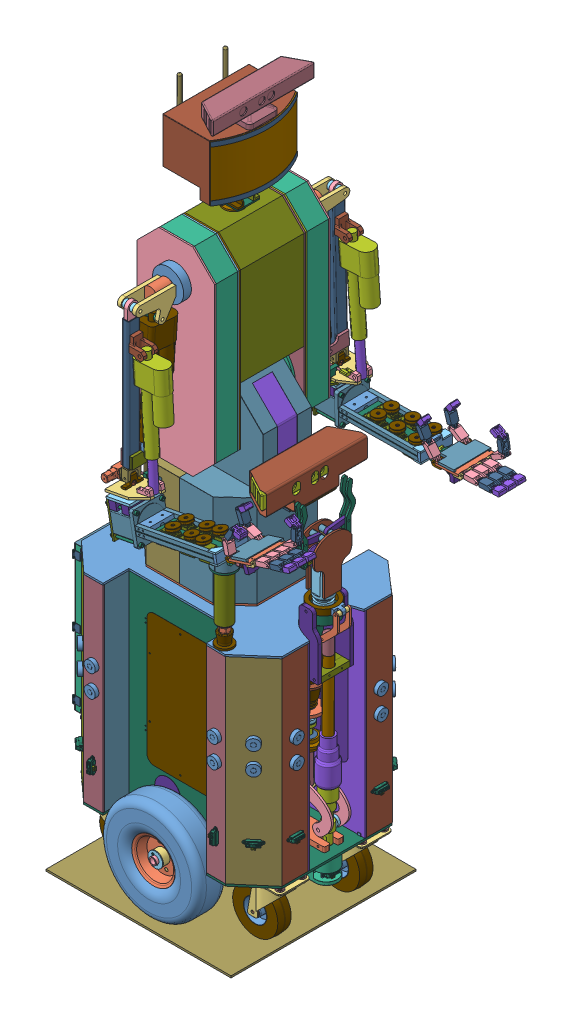
SolidWorks assembly sorbot, configuration По умолчанию. Lengths in mm. (continued)
Components (placement in the parent): (continued)
- man1.drive1-1: man1.drive1 [По умолчанию] at (-119.3768 640.728 -141.6211) x (0.999934 0 -0.01146) z (0 1 0) size (50 50 148.25)
- body.tilit.planetary.drive.fixture.p1-1: body.tilit.planetary.drive.fixture.p1 [По умолчанию] at (-119.3768 612.7934 -141.6211) size (85 10 85)
- body.tilit.planetary.drive.fixture.p2-1: body.tilit.planetary.drive.fixture.p2 [По умолчанию] at (-119.3768 622.7934 -141.6211) size (85 4 85)
- tilt.thread.rod.fixture.2-2: tilt.thread.rod.fixture.2 [По умолчанию] at (-119.3768 793.5591 -141.6211) x (-0.837169 0 -0.546944) z (-0.546944 0 0.837169) size (40 26 40)
- body.tilit.planetary.drive.fixture.p3-1: body.tilit.planetary.drive.fixture.p3 [По умолчанию] at (-119.3768 695.728 -141.6211) size (68 8 68)
- body.tilit.planetary.drive.fixture.p4-1: body.tilit.planetary.drive.fixture.p4 [По умолчанию] at (-119.3768 753.9526 -141.6211) x (0.997546 0 -0.070011) z (0.070011 0 0.997546) size (70 9 70)
- body.tilit.planetary.drive.fixture.p5-1: body.tilit.planetary.drive.fixture.p5 [По умолчанию] at (-148.8664 612.7934 -141.6211) size (5 157 5)
- m6.nut-13: m6.nut [По умолчанию] at (-148.8664 613.2934 -141.6211) size (10 5.5 11.55)
- body.tilit.planetary.drive.fixture.p5-2: body.tilit.planetary.drive.fixture.p5 [По умолчанию] at (-89.8872 612.7934 -141.6211) size (5 157 5)
- body.tilit.planetary.drive.fixture.p5-3: body.tilit.planetary.drive.fixture.p5 [По умолчанию] at (-119.3768 612.7934 -112.1315) size (5 157 5)
- body.tilit.planetary.drive.fixture.p5-4: body.tilit.planetary.drive.fixture.p5 [По умолчанию] at (-119.3768 612.7934 -171.1107) size (5 157 5)
- m6.nut-14: m6.nut [По умолчанию] at (-89.8872 613.2934 -141.6211) size (10 5.5 11.55)
- m6.nut-15: m6.nut [По умолчанию] at (-119.3768 613.2934 -171.1107) x (0.598875 0 -0.800843) z (0.800843 0 0.598875) size (10 5.5 11.55)
- m6.nut-16: m6.nut [По умолчанию] at (-119.3768 613.2934 -112.1315) x (-0.286054 0 -0.958214) z (0.958214 0 -0.286054) size (10 5.5 11.55)
- m6.nut-17: m6.nut [По умолчанию] at (-119.3768 768.4526 -112.1315) x (-0.837169 0 -0.546944) z (-0.546944 0 0.837169) size (10 5.5 11.55)
- m6.nut-18: m6.nut [По умолчанию] at (-89.8872 768.4526 -141.6211) x (-0.837169 0 -0.546944) z (-0.546944 0 0.837169) size (10 5.5 11.55)
- m6.nut-19: m6.nut [По умолчанию] at (-119.3768 768.4526 -171.1107) x (-0.837169 0 -0.546944) z (-0.546944 0 0.837169) size (10 5.5 11.55)
- m6.nut-20: m6.nut [По умолчанию] at (-148.8664 768.4526 -141.6211) x (-0.837169 0 -0.546944) z (-0.546944 0 0.837169) size (10 5.5 11.55)
- m6.nut-21: m6.nut [По умолчанию] at (-29.5996 1324.99 9.9014) x (-0.526603 0.850111 0) z (0 0 1) size (10 5.5 11.55)
- m6.6.50mm-1: m6.6.50mm [По умолчанию] at (4.3029 1345.9909 9.9014) x (0.525089 -0.847668 0.075763) z (-0.039897 0.064407 0.997126) size (10 56 10)
- m4.nut-1: m4.nut [По умолчанию] at (-35.3987 1340.8364 4.6679) x (1 0 0) z (0 -1 0) size (6.86 5 7.92)
- m4.nut-2: m4.nut [По умолчанию] at (-103.2224 997.8992 -35.7442) x (1 0 0) z (0 -1 0) size (6.86 5 7.92)
- arm.rotate-1: arm.rotate [По умолчанию] at (22.4782 854.2475 144.4763) x (0 0 1) z (-0.185706 0.982605 0) size (85.26 111.5 91.5)
  - SY85STH65-2808A-1: SY85STH65-2808A [По умолчанию] at (-4.2017 8.56 0) size (85.26 96.5 85)
  - m6.6.80mm-1: m6.6.80mm [По умолчанию] at (-39.0017 18.56 -34.8) size (10 86 10)
  - m6.6.80mm-2: m6.6.80mm [По умолчанию] at (30.5983 18.56 34.8) size (10 86 10)
  - m6.6.80mm-3: m6.6.80mm [По умолчанию] at (30.5983 18.56 -34.8) size (10 86 10)
  - m6.6.80mm-4: m6.6.80mm [По умолчанию] at (-39.0017 18.56 34.8) size (10 86 10)
  - arm.rotate.p2-2: arm.rotate.p2 [По умолчанию] at (-46.7017 -46.44 42.5) x (1 0 0) z (0 -1 0) size (85 91.5 5)
  - m6.nut-1: m6.nut [По умолчанию] at (30.5983 -56.94 34.8) size (10 5.5 11.55)
  - m6.nut-2: m6.nut [По умолчанию] at (-39.0017 -56.94 -34.8) size (10 5.5 11.55)
  - m6.nut-3: m6.nut [По умолчанию] at (-39.0017 -56.94 34.8) size (10 5.5 11.55)
  - m6.nut-4: m6.nut [По умолчанию] at (30.5983 -56.94 -34.8) size (10 5.5 11.55)
  - arm.rotate.p1-2: arm.rotate.p1 [По умолчанию] at (-4.2017 8.56 38) x (1 0 0) z (0 -1 0) size (85 21 20)
  - arm.rotate.p1-3: arm.rotate.p1 [По умолчанию] at (-4.2017 -26.44 38) x (1 0 0) z (0 -1 0) size (85 21 20)
- arm.rotate.p8-1: arm.rotate.p8 [По умолчанию] at (-48.9081 912.5039 130.5417) x (-0.185706 0.982605 0) z (0 0 1) size (25 12 48)
- arm.rotate.p9-1: arm.rotate.p9 [По умолчанию] at (42.4949 859.0482 172.7746) x (0.982605 0.185706 0) z (0 0 1) size (30 10 65)
- arm.rotate.p9-2: arm.rotate.p9 [По умолчанию] at (72.3444 862.6542 172.7746) x (-0.982605 -0.185706 0) z (0 0 1) size (30 10 65)
- arm.elbow.rotate.p1-1: arm.elbow.rotate.p1 [По умолчанию] at (-55.7977 924.3811 168.7746) x (-0.185706 0.982605 0) z (0 0 -1) size (21.9 27.89 71.5)
- arm.rotate.p6-1: arm.rotate.p6 [По умолчанию] at (20.223 919.4631 140.2746) x (0 0 1) z (-0.982605 -0.185706 0) size (85 6 102)
- arm.rotate.p7-1: arm.rotate.p7 [По умолчанию] at (81.3033 937.1131 170.2746) x (-0.185706 0.982605 0) z (0 0 -1) size (16 36 10)
- arm.rotate.p7-2: arm.rotate.p7 [По умолчанию] at (81.3033 937.1131 140.2746) x (-0.185706 0.982605 0) z (0 0 -1) size (16 36 10)
- arm.rotate.p10-1: arm.rotate.p10 [По умолчанию] at (-37.1666 892.8424 182.7746) x (0 0 -1) z (0.982605 0.185706 0) size (85 6 65)
- arm.elbow.rotate.bearing-1: arm.elbow.rotate.bearing [По умолчанию] at (-7.5173 911.1932 140.056) x (-0.183128 -0.03461 0.98248) z (-0.96539 -0.182453 -0.18637) size (61.4 10 61.4)
  - arm.elbow.rotate.bearing.p1-1: arm.elbow.rotate.bearing.p1 [По умолчанию] at (0.2225 -3.7755 0) size (61.4 4.5 61.4)
  - ball.10mm-1: ball.10mm [По умолчанию] at (0.0947 -1.5255 -24.7664) size (10 10 10)
  - ball.10mm-2: ball.10mm [По умолчанию] at (-9.9677 -1.5255 -22.5733) x (0.913545 0 -0.406737) z (0.406737 0 0.913545) size (10 10 10)
  - ball.10mm-3: ball.10mm [По умолчанию] at (-18.2681 -1.5255 -16.477) x (0.669131 0 -0.743145) z (0.743145 0 0.669131) size (10 10 10)
  - ball.10mm-4: ball.10mm [По умолчанию] at (-23.3713 -1.5255 -7.5317) x (0.309017 0 -0.951057) z (0.951057 0 0.309017) size (10 10 10)
  - ball.10mm-5: ball.10mm [По умолчанию] at (-24.3949 -1.5255 2.7159) x (-0.104528 0 -0.994522) z (0.994522 0 -0.104528) size (10 10 10)
  - ball.10mm-6: ball.10mm [По умолчанию] at (-21.162 -1.5255 12.4939) x (-0.5 0 -0.866025) z (0.866025 0 -0.5) size (10 10 10)
  - ball.10mm-7: ball.10mm [По умолчанию] at (-14.2315 -1.5255 20.1116) x (-0.809017 0 -0.587785) z (0.587785 0 -0.809017) size (10 10 10)
  - ball.10mm-8: ball.10mm [По умолчанию] at (-4.8018 -1.5255 24.2518) x (-0.978148 0 -0.207912) z (0.207912 0 -0.978148) size (10 10 10)
  - ball.10mm-9: ball.10mm [По умолчанию] at (5.4967 -1.5255 24.1987) x (-0.978148 0 0.207912) z (-0.207912 0 -0.978148) size (10 10 10)
  - ball.10mm-10: ball.10mm [По умолчанию] at (14.8832 -1.5255 19.9614) x (-0.809017 0 0.587785) z (-0.587785 0 -0.809017) size (10 10 10)
  - ball.10mm-11: ball.10mm [По умолчанию] at (21.7347 -1.5255 12.2726) x (-0.5 0 0.866025) z (-0.866025 0 -0.5) size (10 10 10)
  - ball.10mm-12: ball.10mm [По умолчанию] at (24.8666 -1.5255 2.4617) x (-0.104528 0 0.994522) z (-0.994522 0 -0.104528) size (10 10 10)
  - ball.10mm-13: ball.10mm [По умолчанию] at (23.7373 -1.5255 -7.7748) x (0.309017 0 0.951057) z (-0.951057 0 0.309017) size (10 10 10)
  - ball.10mm-14: ball.10mm [По умолчанию] at (18.542 -1.5255 -16.6669) x (0.669131 0 0.743145) z (-0.743145 0 0.669131) size (10 10 10)
  - ball.10mm-15: ball.10mm [По умолчанию] at (10.1792 -1.5255 -22.6772) x (0.913545 0 0.406737) z (-0.406737 0 0.913545) size (10 10 10)
- arm.elbow.rotate.p3-1: arm.elbow.rotate.p3 [По умолчанию] at (-6.3462 904.7735 140.2746) x (0.982605 0.185706 0) z (0 0 1) size (36.4 9 36.4)
- arm.elbow.rotate.p4-1: arm.elbow.rotate.p4 [По умолчанию] at (-6.3462 904.7735 140.2746) x (0.982605 0.185706 0) z (0 0 1) size (22 7 22)
- bolt.m8.short-1: bolt.m8.short [По умолчанию] at (-3.7463 891.017 140.2746) x (0.982605 0.185706 0) z (0 0 1) size (12.8 43 12.8)
- m8.nut-1: m8.nut [По умолчанию] at (-9.2247 920.0039 140.2746) x (0.979774 0.185171 -0.075859) z (0.07454 0.014088 0.997119) size (14.97 7 13.53)
- arm.rotate.p11-1: arm.rotate.p11 [По умолчанию] at (-41.1593 913.9684 141.7746) x (-0.185706 0.982605 0) z (0 0 -1) size (24 14 44)
- arm.elbow.rotate.p5-1: arm.elbow.rotate.p5 [По умолчанию] at (-37.816 927.7795 114.7746) x (-0.0817 0.432291 -0.898025) z (0.982605 0.185706 0) size (5 5 75)
- arm.elbow.rotate.p6-1: arm.elbow.rotate.p6 [По умолчанию] at (39.7316 938.238 120.2746) x (0 0 1) z (-0.982685 -0.185282 0) size (21 8 17.99)
- arm.elbow.rotate.p11-1: arm.elbow.rotate.p11 [По умолчанию] at (-1.3122 934.6785 114.7746) x (0 0 -1) z (0.982605 0.185706 0) size (29.5 27.93 10)
- arm.elbow.rotate.p12-1: arm.elbow.rotate.p12 [По умолчанию] at (0.0407 905.9806 81.7746) x (0.589563 0.111424 0.8) z (-0.786084 -0.148565 0.6) size (29 4.5 14)
- arm.elbow.rotate.p13-1: arm.elbow.rotate.p13 [По умолчанию] at (-28.3338 929.5716 114.7746) x (-0.185706 0.982605 0) z (0 0 1) size (9 12 9)
- arm.elbow.rotate.p14-1: arm.elbow.rotate.p14 [По умолчанию] at (-41.599 927.0645 114.7746) x (0 0 -1) z (0.982605 0.185706 0) size (18 18 10)
- palm.tilt.p1-1: palm.tilt.p1 [По умолчанию] at (76.6621 839.8086 140.4246) x (0.185706 -0.982605 0) z (0 0 1) size (36.5 37.1 24.8)
- palm.drives.fixture-2: palm.drives.fixture [По умолчанию] at (72.6077 850.4915 150.4246) x (0.982605 0.185706 0) z (0 0 -1) size (30.05 15 65)
- palm.lift.p2-2: palm.lift.p2 [По умолчанию] at (97.1945 857.1737 140.4246) x (0.033136 -0.175327 -0.983952) z (0.982605 0.185706 0) size (5 5 158)
- palm.drive.thread.fixture.p2-1: palm.drive.thread.fixture.p2 [По умолчанию] at (87.8616 855.4098 140.4246) x (-0.05957 0.315194 0.947156) z (0.982605 0.185706 0) size (11.8 11.8 25)
- m3x8-1: m3x8 [По умолчанию] at (92.8919 850.6734 142.3172) x (0.982605 0.185707 0) z (0.05957 -0.315194 -0.947156) size (5.3 6.85 5.3)
- m3x8-2: m3x8 [По умолчанию] at (101.0372 852.2128 142.3172) x (0.982605 0.185707 0) z (0.05957 -0.315194 -0.947156) size (5.3 6.85 5.3)
- palm.drive.thread.fixture-1: palm.drive.thread.fixture [По умолчанию] at (254.7288 885.7804 140.4246) x (0 0 -1) z (-0.982605 -0.185706 0) size (30 34 7)
- palm.lift.fixture-1: palm.lift.fixture [По умолчанию] at (260.6332 900.2751 126.1211) x (0 0 -1) z (0.185706 -0.982605 0) size (30 17 12)
- palm.lift.fixture.p2-1: palm.lift.fixture.p2 [По умолчанию] at (287.8736 901.2786 140.2746) x (0 0 1) z (-0.950223 -0.311571 0) size (26 12.5 30)
- PALM.LIFT.THREAD.FIXTURE.P3-1: PALM.LIFT.THREAD.FIXTURE.P3 [По умолчанию] at (131.0658 873.7522 140.2958) x (-0.982605 -0.185706 0) z (0 0 1) size (20 14 10)
- palm.lift.drive.nut-1: palm.lift.drive.nut [По умолчанию] at (168.1531 870.5844 140.4246) x (0.124167 -0.656989 -0.743604) z (0.982605 0.185706 0) size (12 12 16)
- palm.lift.nut.fixture-1: palm.lift.nut.fixture [По умолчанию] at (174.1569 881.8961 145.4246) x (0 0 -1) z (-0.982605 -0.185706 0) size (10 28 10)
- palm.lift.nut.fixture-2: palm.lift.nut.fixture [По умолчанию] at (174.1569 881.8961 135.4246) x (0 0 1) z (0.982605 0.185706 0) size (10 28 10)
- palm.lift.p4-1: palm.lift.p4 [По умолчанию] at (168.591 857.4974 140.4246) x (0 0 -1) z (0.982605 0.185706 0) size (4 4 120)
- palm.lift.fixture.p6-1: palm.lift.fixture.p6 [По умолчанию] at (276.6776 877.9252 140.4246) x (0 0 -1) z (0.982605 0.185706 0) size (12 12 20.44)
- palm.lift.fixture.p7-1: palm.lift.fixture.p7 [По умолчанию] at (292.1321 880.846 138.4246) x (0.730069 0.683374 0) z (0 0 1) size (27 9 4)
- m6.washer-1: m6.washer [По умолчанию] at (284.4317 914.5677 140.506) x (0.950223 0.311571 0.000222) z (-0.000211 -0.000069 1) size (18 1.7 18)
- m6.washer-2: m6.washer [По умолчанию] at (289.4791 899.1741 140.506) x (-0.950223 -0.311571 -0.000219) z (-0.000208 -0.000068 1) size (18 1.7 18)
- m6.washer-3: m6.washer [По умолчанию] at (286.8308 907.251 140.506) x (0.950223 0.311571 0.000222) z (-0.000211 -0.000069 1) size (18 1.7 18)
- palm.lift.on-palm.fixture-2: palm.lift.on-palm.fixture [По умолчанию] at (300.1799 895.8423 140.2746) x (0 0 -1) z (0.950223 0.311571 0) size (26 23.89 8)
- palm.lift.p1-1: palm.lift.p1 [По умолчанию] at (338.412 919.9816 174.4917) x (0.950144 0.311545 0.012888) z (-0.311571 0.950223 0) size (36.5 37.1 24.8)
- palm.drive.thread.fixture.p2-2: palm.drive.thread.fixture.p2 [По умолчанию] at (325.9934 915.9097 160.372) x (-0.999321 0.034794 -0.0121) z (0.012247 0.004016 -0.999917) size (11.8 11.8 25)
- palm.tilit.fixture-1: palm.tilit.fixture [По умолчанию] at (336.6565 929.587 176.5089) x (0.012247 0.004016 -0.999917) z (-0.950144 -0.311545 -0.012888) size (12 17 18)
- palm.tilit.p8-1: palm.tilit.p8 [По умолчанию] at (326.1771 915.9699 145.3733) x (-0.999829 0.013918 -0.01219) z (0.012247 0.004016 -0.999917) size (5 5 57)
- palm.tilit.p9-1: palm.tilit.p9 [По умолчанию] at (336.3842 931.6025 91.2066) x (-0.950144 -0.311545 -0.012888) z (-0.012247 -0.004016 0.999917) size (23.81 15.6 6)
- palm.tilit.p10-1: palm.tilit.p10 [По умолчанию] at (303.1082 912.5882 153.2746) x (0 0 -1) z (0.950223 0.311571 0) size (26 8.5 15)
- palm.tilit.p11-1: palm.tilit.p11 [По умолчанию] at (326.5434 916.09 115.4643) x (0.950144 0.311545 0.012888) z (-0.012247 -0.004016 0.999917) size (17.95 8 10)
- palm.tilit.p12-1: palm.tilit.p12 [По умолчанию] at (317.7933 904.2485 140.2746) x (0.070018 0.022958 -0.997282) z (0.94764 0.310724 0.073685) size (29 4 9)
- arm.rotate.p6-2: arm.rotate.p6 [По умолчанию] at (17.2833 914.2431 -421.887) x (-0.005195 -0.022106 0.999742) z (-0.99991 -0.012267 -0.005467) size (85 6 102)
- arm.rotate.p8-2: arm.rotate.p8 [По умолчанию] at (-52.6122 919.605 -432.1343) x (-0.012385 0.99968 0.022041) z (-0.005195 -0.022106 0.999742) size (25 12 48)
- arm.rotate.p7-3: arm.rotate.p7 [По умолчанию] at (80.4988 921.0176 -421.4088) x (-0.012385 0.99968 0.022041) z (0.005195 0.022106 -0.999742) size (16 36 10)
- arm.rotate.p7-4: arm.rotate.p7 [По умолчанию] at (80.343 920.3544 -391.4165) x (-0.012385 0.99968 0.022041) z (0.005195 0.022106 -0.999742) size (16 36 10)
- bolt.m8.short-2: bolt.m8.short [По умолчанию] at (-11.2814 892.2812 -422.5211) x (0.999923 0.012406 -0.000807) z (0.00108 -0.022029 0.999757) size (12.8 43 12.8)
- m8.nut-2: m8.nut [По умолчанию] at (-11.6234 919.8874 -421.9124) x (0.559915 -0.011329 0.828472) z (-0.828457 -0.022602 0.559596) size (14.97 7 13.53)
- arm.elbow.rotate.bearing-2: arm.elbow.rotate.bearing [По умолчанию] at (-11.6907 910.4164 -422.2454) x (0.829913 -0.002018 0.557889) z (-0.557755 -0.025201 0.829623) size (61.4 10 61.4)
  - arm.elbow.rotate.bearing.p1-1: arm.elbow.rotate.bearing.p1 [По умолчанию] at (0.2225 -3.7755 0) size (61.4 4.5 61.4)
  - ball.10mm-1: ball.10mm [По умолчанию] at (0.0947 -1.5255 -24.7664) size (10 10 10)
  - ball.10mm-2: ball.10mm [По умолчанию] at (-9.9677 -1.5255 -22.5733) x (0.913545 0 -0.406737) z (0.406737 0 0.913545) size (10 10 10)
  - ball.10mm-3: ball.10mm [По умолчанию] at (-18.2681 -1.5255 -16.477) x (0.669131 0 -0.743145) z (0.743145 0 0.669131) size (10 10 10)
  - ball.10mm-4: ball.10mm [По умолчанию] at (-23.3713 -1.5255 -7.5317) x (0.309017 0 -0.951057) z (0.951057 0 0.309017) size (10 10 10)
  - ball.10mm-5: ball.10mm [По умолчанию] at (-24.3949 -1.5255 2.7159) x (-0.104528 0 -0.994522) z (0.994522 0 -0.104528) size (10 10 10)
  - ball.10mm-6: ball.10mm [По умолчанию] at (-21.162 -1.5255 12.4939) x (-0.5 0 -0.866025) z (0.866025 0 -0.5) size (10 10 10)
  - ball.10mm-7: ball.10mm [По умолчанию] at (-14.2315 -1.5255 20.1116) x (-0.809017 0 -0.587785) z (0.587785 0 -0.809017) size (10 10 10)
  - ball.10mm-8: ball.10mm [По умолчанию] at (-4.8018 -1.5255 24.2518) x (-0.978148 0 -0.207912) z (0.207912 0 -0.978148) size (10 10 10)
  - ball.10mm-9: ball.10mm [По умолчанию] at (5.4967 -1.5255 24.1987) x (-0.978148 0 0.207912) z (-0.207912 0 -0.978148) size (10 10 10)
  - ball.10mm-10: ball.10mm [По умолчанию] at (14.8832 -1.5255 19.9614) x (-0.809017 0 0.587785) z (-0.587785 0 -0.809017) size (10 10 10)
  - ball.10mm-11: ball.10mm [По умолчанию] at (21.7347 -1.5255 12.2726) x (-0.5 0 0.866025) z (-0.866025 0 -0.5) size (10 10 10)
  - ball.10mm-12: ball.10mm [По умолчанию] at (24.8666 -1.5255 2.4617) x (-0.104528 0 0.994522) z (-0.994522 0 -0.104528) size (10 10 10)
  - ball.10mm-13: ball.10mm [По умолчанию] at (23.7373 -1.5255 -7.7748) x (0.309017 0 0.951057) z (-0.951057 0 0.309017) size (10 10 10)
  - ball.10mm-14: ball.10mm [По умолчанию] at (18.542 -1.5255 -16.6669) x (0.669131 0 0.743145) z (-0.743145 0 0.669131) size (10 10 10)
  - ball.10mm-15: ball.10mm [По умолчанию] at (10.1792 -1.5255 -22.6772) x (0.913545 0 0.406737) z (-0.406737 0 0.913545) size (10 10 10)
- arm.elbow.rotate.p4-2: arm.elbow.rotate.p4 [По умолчанию] at (-11.4253 903.8925 -422.2651) x (0.756023 0.023788 -0.654112) z (0.654428 -0.008562 0.756076) size (22 7 22)
- arm.elbow.rotate.p3-2: arm.elbow.rotate.p3 [По умолчанию] at (-11.4253 903.8925 -422.2651) x (0.999923 0.012396 -0.000381) z (0.000654 -0.022034 0.999757) size (36.4 9 36.4)
- arm.rotate.p10-2: arm.rotate.p10 [По умолчанию] at (-43.7015 904.4334 -464.9318) x (-0.005195 -0.022106 0.999742) z (0.99991 0.012267 0.005467) size (85 6 65)
- arm.rotate-2: arm.rotate [По умолчанию] at (8.1724 849.0496 -419.1732) x (-0.005195 -0.022106 0.999742) z (-0.012385 0.99968 0.022041) size (85.26 111.5 91.5)
  - SY85STH65-2808A-1: SY85STH65-2808A [По умолчанию] at (-4.2017 8.56 0) size (85.26 96.5 85)
  - m6.6.80mm-1: m6.6.80mm [По умолчанию] at (-39.0017 18.56 -34.8) size (10 86 10)
  - m6.6.80mm-2: m6.6.80mm [По умолчанию] at (30.5983 18.56 34.8) size (10 86 10)
  - m6.6.80mm-3: m6.6.80mm [По умолчанию] at (30.5983 18.56 -34.8) size (10 86 10)
  - m6.6.80mm-4: m6.6.80mm [По умолчанию] at (-39.0017 18.56 34.8) size (10 86 10)
  - arm.rotate.p2-2: arm.rotate.p2 [По умолчанию] at (-46.7017 -46.44 42.5) x (1 0 0) z (0 -1 0) size (85 91.5 5)
  - m6.nut-1: m6.nut [По умолчанию] at (30.5983 -56.94 34.8) size (10 5.5 11.55)
  - m6.nut-2: m6.nut [По умолчанию] at (-39.0017 -56.94 -34.8) size (10 5.5 11.55)
  - m6.nut-3: m6.nut [По умолчанию] at (-39.0017 -56.94 34.8) size (10 5.5 11.55)
  - m6.nut-4: m6.nut [По умолчанию] at (30.5983 -56.94 -34.8) size (10 5.5 11.55)
  - arm.rotate.p1-2: arm.rotate.p1 [По умолчанию] at (-4.2017 8.56 38) x (1 0 0) z (0 -1 0) size (85 21 20)
  - arm.rotate.p1-3: arm.rotate.p1 [По умолчанию] at (-4.2017 -26.44 38) x (1 0 0) z (0 -1 0) size (85 21 20)
- arm.rotate.p9-3: arm.rotate.p9 [По умолчанию] at (59.0931 848.0507 -390.6251) x (-0.99991 -0.012267 -0.005467) z (-0.005195 -0.022106 0.999742) size (30 10 65)
- arm.rotate.p9-4: arm.rotate.p9 [По умолчанию] at (29.0711 849.682 -390.745) x (0.99991 0.012267 0.005467) z (-0.005195 -0.022106 0.999742) size (30 10 65)
- arm.rotate.p11.mirr-1: arm.rotate.p11.mirr [По умолчанию] at (-44.3413 918.5492 -379.6011) x (-0.012385 0.99968 0.022041) z (0.005195 0.022106 -0.999742) size (24 14 44)
- arm.elbow.rotate.p1-2: arm.elbow.rotate.p1 [По умолчанию] at (-56.5709 932.0381 -450.3776) x (0.012299 -0.999907 -0.005858) z (-0.005395 -0.005924 0.999968) size (21.9 27.89 71.5)
- arm.elbow.rotate.p6.mirr-1: arm.elbow.rotate.p6.mirr [По умолчанию] at (20.3416 928.6659 -401.5471) x (0.005195 0.022106 -0.999742) z (0.99991 0.012267 0.005467) size (21 8 17.99)
- arm.elbow.rotate.p13-2: arm.elbow.rotate.p13 [По умолчанию] at (-28.5648 932.0653 -396.2246) x (0.012299 -0.999907 -0.005858) z (0.005395 0.005924 -0.999968) size (9 12 9)
- arm.elbow.rotate.p14-2: arm.elbow.rotate.p14 [По умолчанию] at (-42.4135 931.8954 -396.3003) x (0.005872 -0.033224 -0.999431) z (0.99991 0.012267 0.005467) size (18 18 10)
- arm.elbow.rotate.p5-2: arm.elbow.rotate.p5 [По умолчанию] at (-38.5639 931.9427 -396.2793) x (0.005872 -0.033224 -0.999431) z (0.99991 0.012267 0.005467) size (5 5 75)
- arm.elbow.rotate.p11-2: arm.elbow.rotate.p11 [По умолчанию] at (8.5819 932.5211 -396.0215) x (-0.005195 -0.022106 0.999742) z (-0.99991 -0.012267 -0.005467) size (29.5 27.93 10)
- arm.elbow.rotate.p12-2: arm.elbow.rotate.p12 [По умолчанию] at (-5.2424 903.6993 -363.7222) x (0.604102 0.025046 -0.796513) z (0.796811 -0.00345 0.604219) size (29 4.5 14)
- palm.drives.fixture-3: palm.drives.fixture [По умолчанию] at (57.358 836.5241 -413.2447) x (0.99991 0.012267 0.005467) z (0.005195 0.022106 -0.999742) size (30.05 15 65)
- palm.tilt.p1-2: palm.tilt.p1 [По умолчанию] at (59.5491 825.5233 -423.4792) x (0.012385 -0.99968 -0.022041) z (-0.005195 -0.022106 0.999742) size (36.5 37.1 24.8)
- palm.drive.thread.fixture.p2-3: palm.drive.thread.fixture.p2 [По умолчанию] at (73.3338 838.9402 -423.1109) x (0.002801 0.207624 -0.978205) z (0.99991 0.012267 0.005467) size (11.8 11.8 25)
- palm.lift.p2-3: palm.lift.p2 [По умолчанию] at (85.2879 839.0868 -423.0455) x (0.006111 -0.053098 -0.998571) z (0.99991 0.012267 0.005467) size (5 5 158)
- palm.lift.drive.nut-2: palm.lift.drive.nut [По умолчанию] at (152.3766 839.9099 -422.6787) x (-0.003006 -0.192356 0.981321) z (0.99991 0.012267 0.005467) size (12 12 16)
- palm.lift.nut.fixture-3: palm.lift.nut.fixture [По умолчанию] at (160.2261 849.8943 -417.4158) x (0.005195 0.022106 -0.999742) z (-0.99991 -0.012267 -0.005467) size (10 28 10)
- palm.lift.nut.fixture-4: palm.lift.nut.fixture [По умолчанию] at (160.278 850.1154 -427.4132) x (-0.005195 -0.022106 0.999742) z (0.99991 0.012267 0.005467) size (10 28 10)
- palm.lift.p4-2: palm.lift.p4 [По умолчанию] at (150.9783 826.9543 -422.9724) x (-0.009526 0.934752 -0.355174) z (0.99991 0.012267 0.005467) size (4 4 120)
- palm.lift.fixture-2: palm.lift.fixture [По умолчанию] at (251.2934 853.4367 -436.1728) x (0.005195 0.022106 -0.999742) z (0.012385 -0.99968 -0.022041) size (30 17 12)
- palm.lift.fixture.p2-2: palm.lift.fixture.p2 [По умолчанию] at (278.3444 848.1669 -421.9915) x (-0.005195 -0.022106 0.999742) z (-0.998179 -0.059975 -0.006513) size (26 12.5 30)
- palm.drive.thread.fixture-2: palm.drive.thread.fixture [По умолчанию] at (243.3826 839.8806 -422.2064) x (0.005195 0.022106 -0.999742) z (-0.99991 -0.012267 -0.005467) size (30 34 7)
- m6.washer-4: m6.washer [По умолчанию] at (279.3618 845.7191 -421.8089) x (-0.988782 -0.062508 0.135656) z (0.136738 -0.013357 0.990517) size (18 1.7 18)
- m6.washer-5: m6.washer [По умолчанию] at (278.8509 854.2017 -421.624) x (-0.923349 -0.063864 0.378614) z (-0.379229 -0.002669 -0.925299) size (18 1.7 18)
- m6.washer-6: m6.washer [По умолчанию] at (278.3881 861.886 -421.4565) x (-0.923349 -0.063864 0.378614) z (-0.379229 -0.002669 -0.925299) size (18 1.7 18)
- palm.lift.fixture.p6-2: palm.lift.fixture.p6 [По умолчанию] at (260.9684 828.3037 -422.371) x (0.005195 0.022106 -0.999742) z (0.99991 0.012267 0.005467) size (12 12 20.44)
- palm.lift.on-palm.fixture-3: palm.lift.on-palm.fixture [По умолчанию] at (288.8671 839.7851 -422.1222) x (0.005195 0.022106 -0.999742) z (0.998179 0.059975 0.006513) size (26 23.89 8)
- palm.lift.fixture.p7-2: palm.lift.fixture.p7 [По умолчанию] at (276.6855 828.4557 -420.4355) x (0.911851 0.41029 0.013811) z (0.005195 0.022106 -0.999742) size (27 9 4)
- palm.tilit.fixture-2: palm.tilit.fixture [По умолчанию] at (333.8862 862.4481 -385.8466) x (0.005195 0.022106 -0.999742) z (-0.998179 -0.059975 -0.006513) size (12 17 18)
- palm.lift.p1-2: palm.lift.p1 [По умолчанию] at (332.7336 852.6936 -388.0688) x (0.998179 0.059975 0.006513) z (-0.060104 0.997955 0.021755) size (36.5 37.1 24.8)
- palm.drive.thread.fixture.p2-4: palm.drive.thread.fixture.p2 [По умолчанию] at (319.5802 852.2073 -402.1015) x (0.991144 0.132548 0.008081) z (0.005195 0.022106 -0.999742) size (11.8 11.8 25)
- palm.tilit.p8-2: palm.tilit.p8 [По умолчанию] at (319.9542 853.799 -474.0829) x (0.998896 -0.046783 0.004156) z (-0.005195 -0.022106 0.999742) size (5 5 57)
- palm.tilit.p9-2: palm.tilit.p9 [По умолчанию] at (333.0838 866.2226 -471.0893) x (-0.998179 -0.059975 -0.006513) z (-0.005195 -0.022106 0.999742) size (23.81 15.6 6)
- palm.tilit.p10-2: palm.tilit.p10 [По умолчанию] at (295.8835 854.9468 -408.7471) x (0.005195 0.022106 -0.999742) z (0.998179 0.059975 0.006513) size (26 8.5 15)
- palm.tilit.p12-2: palm.tilit.p12 [По умолчанию] at (308.0373 843.4408 -421.9418) x (0.090521 0.027153 -0.995524) z (0.994079 0.057865 0.091968) size (29 4 9)
- palm.tilit.p11-2: palm.tilit.p11 [По умолчанию] at (319.8114 853.1912 -446.5982) x (0.998179 0.059975 0.006513) z (-0.005195 -0.022106 0.999742) size (17.95 8 10)
- SY57STH56-2804A-1: SY57STH56-2804A [Default] at (-12.4903 1378.2936 -136.5542) x (1 0 0) z (0 0 1) size (56 76.6 56)
- head.tilt.p1-1: head.tilt.p1 [По умолчанию] at (-12.4903 1438.7936 -136.5542) x (0.436164 0 -0.899867) z (0.899867 0 0.436164) size (54 17.5 54)
- head.rotate.bearing-1: head.rotate.bearing [По умолчанию] at (-12.4903 1435.8936 -136.5542) x (1 0 0) z (0 0 1) size (30 8.9 30)
- head.rotate.bearing.insert-1: head.rotate.bearing.insert [По умолчанию] at (-12.4903 1435.8936 -136.5542) x (1 0 0) z (0 0 1) size (17 8.5 17)
- SY42STH47-1: SY42STH47 [Default] at (-33.8403 1484.4436 -199.0542) x (-1 0 0) z (0 1 0) size (42.3 80.5 42.3)
- head.tilt.p2-1: head.tilt.p2 [По умолчанию] at (-33.8403 1484.4436 -144.3542) x (-0.997593 -0.06934 0) z (-0.06934 0.997593 0) size (15 9.8 14.97)
- head.tilit.p4-1: head.tilit.p4 [По умолчанию] at (-2.6766 1441.2936 -156.8012) x (1 0 0) z (0 0 1) size (9.2 13.5 9.2)
- head.tilit.p4-2: head.tilit.p4 [По умолчанию] at (7.7567 1441.2936 -126.7405) x (1 0 0) z (0 0 1) size (9.2 13.5 9.2)
- head.tilit.p4-3: head.tilit.p4 [По умолчанию] at (-22.304 1441.2936 -116.3072) x (1 0 0) z (0 0 1) size (9.2 13.5 9.2)
- head.tilit.p4-4: head.tilit.p4 [По умолчанию] at (-32.7373 1441.2936 -146.3679) x (1 0 0) z (0 0 1) size (9.2 13.5 9.2)
- head.p1-1: head.p1 [По умолчанию] at (-12.4903 1454.7936 -136.5542) x (0 0 -1) z (1 0 0) size (58.13 3.5 85)
- head.tilit.p5-1: head.tilit.p5 [По умолчанию] at (-54.9903 1463.2936 -152.0542) x (0 0 -1) z (1 0 0) size (16 47.3 85)
- head.tilt.p8-1: head.tilt.p8 [По умолчанию] at (-4.1768 1486.067 -139.0542) x (-0.002177 0.999998 0) z (0.999998 0.002177 0) size (45.99 8.9 45.99)
- head.tilit.p5.m-1: head.tilit.p5.m [По умолчанию] at (30.0097 1463.2936 -117.9254) x (0 0 1) z (-1 0 0) size (16 47.3 85)
- head.tilt.p10-1: head.tilt.p10 [По умолчанию] at (-4.1768 1486.067 -141.5542) x (0.999434 0.033636 0) z (0.033636 -0.999434 0) size (36 3.5 36)
- head.tilt.p10-2: head.tilt.p10 [По умолчанию] at (-4.1768 1486.067 -131.6542) x (0.999434 0.033636 0) z (-0.033636 0.999434 0) size (36 3.5 36)
- head.tilit.p11-1: head.tilit.p11 [По умолчанию] at (-4.1768 1486.067 -131.6542) x (0.999434 0.033636 0) z (0.033636 -0.999434 0) size (36 3.5 113)
- head.tilit.p11-2: head.tilit.p11 [По умолчанию] at (-4.1768 1486.067 -145.0542) x (0.999434 0.033636 0) z (0.033636 -0.999434 0) size (36 3.5 113)
- m4.nut-3: m4.nut [По умолчанию] at (4.9956 1495.2794 -123.1542) x (1 0 0) z (0 1 0) size (6.86 5 7.92)
- m4.nut-4: m4.nut [По умолчанию] at (-4.2051 1499.067 -123.1542) x (1 0 0) z (0 1 0) size (6.86 5 7.92)
- m4.nut-5: m4.nut [По умолчанию] at (5.0356 1476.8947 -123.1542) x (1 0 0) z (0 1 0) size (6.86 5 7.92)
- m4.nut-6: m4.nut [По умолчанию] at (-4.1485 1473.067 -123.1542) x (1 0 0) z (0 1 0) size (6.86 5 7.92)
- m4.nut-7: m4.nut [По умолчанию] at (-13.3492 1476.8546 -123.1542) x (1 0 0) z (0 1 0) size (6.86 5 7.92)
- head.tilt.p12-2: head.tilt.p12 [По умолчанию] at (-4.1768 1486.067 -148.0542) x (1 0 0) z (0 0 1) size (18 18 3)
- m4.nut-8: m4.nut [По умолчанию] at (-13.3892 1495.2394 -123.1542) x (1 0 0) z (0 1 0) size (6.86 5 7.92)
- head.tilt.p9-1: head.tilt.p9 [По умолчанию] at (-4.1768 1486.067 -157.7074) x (0.92329 -0.384104 0) z (0 0 1) size (6 6 45)
- m6.washer-7: m6.washer [По умолчанию] at (-4.1768 1486.067 -117.9254) x (1 0 0) z (0 -1 0) size (18 1.7 18)
- m6.washer-8: m6.washer [По умолчанию] at (-4.1768 1486.067 -152.0542) x (1 0 0) z (0 1 0) size (18 1.7 18)
- head.tilt.p12.m-1: head.tilt.p12.m [По умолчанию] at (-4.1768 1486.067 -128.1542) x (1 0 0) z (0 0 1) size (18 18 6.5)
- head.tilt.p13-1: head.tilt.p13 [По умолчанию] at (-6.8677 1566.0217 -131.6542) x (1 0 0) z (0 1 0) size (30 9.9 30) (hidden)
- head.p3-1: head.p3 [По умолчанию] at (8.1323 1551.1571 -126.1542) x (0 0 1) z (-1 0 0) size (14 31.97 30)
- head.p3-2: head.p3 [По умолчанию] at (-21.8677 1551.1571 -147.0542) x (0 0 -1) z (1 0 0) size (14 31.97 30)
- head.p2-1: head.p2 [По умолчанию] at (-6.6891 1547.1571 -136.5542) x (0 0 -1) z (1 0 0) size (154.89 2 65.43)
- logitech.sphere.af-1: logitech.sphere.af [По умолчанию] at (23.3461 1596.1571 -74.1093) x (0 0 -1) z (1 0 0) size (77.78 90.89 77.78)
- logitech.sphere.af-2: logitech.sphere.af [По умолчанию] at (23.3461 1596.1571 -198.999) x (0 0 -1) z (1 0 0) size (77.78 90.89 77.78)
- head.glass-1: head.glass [По умолчанию] at (-15.5992 1517.1571 -268.7053) x (0.000076 0 1) z (-1 0 0.000076) size (235 150 37.51)
- head.glass.fixture-1: head.glass.fixture [По умолчанию] at (76.9123 1529.1571 -118.3804) x (-0.000076 0 -1) z (0 -1 0) size (235.55 35.5 12)
- head.glass.fixture-2: head.glass.fixture [По умолчанию] at (76.9123 1667.1571 -118.3804) x (-0.000076 0 -1) z (0 -1 0) size (235.55 35.5 12)
- head.p4-1: head.p4 [По умолчанию] at (73.3132 1518.1571 -118.364) x (0 0 -1) z (0 -1 0) size (233.94 161.62 151)
- ant-2: ant [По умолчанию] at (-84.6104 1643.7707 -198.1028) x (0 0 1) z (-1 0 0) size (10 94.18 17)
- ant-3: ant [По умолчанию] at (-84.6104 1643.7707 -74.539) x (0 0 1) z (-1 0 0) size (10 94.18 17)
- kinect-black-1: kinect-black [По умолчанию] at (68.8437 1721.1571 -136.5839) x (0 0 1) z (-1 0 0) size (276 72 65)
- body.cover-1: body.cover [По умолчанию] at (14.9352 1082.7934 -136.9555) x (0 0 -1) z (1 0 0) size (278.72 470.5 152.62)
- Sharp IR GP2D120-1: Sharp IR GP2D120 [Predeterminado] at (274.1242 154.5948 -19.6866) x (0 0 1) z (1 0 0) size (44.5 19 13.9)
  - Sharp IR Body-1: Sharp IR Body [Predeterminado] at (-3.237 2.158 -6.95) size (44.5 13 13.9)
  - Sharp IR JST-1: Sharp IR JST [Predeterminado] at (-3.237 2.158 -3.95) size (28 18 7)
- Sharp IR GP2D120-2: Sharp IR GP2D120 [Predeterminado] at (274.1239 154.5948 -247.6941) x (0 0 1) z (1 0 0) size (44.5 19 13.9)
  - Sharp IR Body-1: Sharp IR Body [Predeterminado] at (-3.237 2.158 -6.95) size (44.5 13 13.9)
  - Sharp IR JST-1: Sharp IR JST [Predeterminado] at (-3.237 2.158 -3.95) size (28 18 7)
- Sharp IR GP2D120-3: Sharp IR GP2D120 [Predeterminado] at (233.0328 154.5948 -324.1002) x (0.759435 0 0.650583) z (0.650583 0 -0.759435) size (44.5 19 13.9)
  - Sharp IR Body-1: Sharp IR Body [Predeterminado] at (-3.237 2.158 -6.95) size (44.5 13 13.9)
  - Sharp IR JST-1: Sharp IR JST [Predeterminado] at (-3.237 2.158 -3.95) size (28 18 7)
- Sharp IR GP2D120-4: Sharp IR GP2D120 [Predeterminado] at (227.8323 154.5948 54.8038) x (-0.759435 0 0.650583) z (0.650583 0 0.759435) size (44.5 19 13.9)
  - Sharp IR Body-1: Sharp IR Body [Predeterminado] at (-3.237 2.158 -6.95) size (44.5 13 13.9)
  - Sharp IR JST-1: Sharp IR JST [Predeterminado] at (-3.237 2.158 -3.95) size (28 18 7)
- Sharp IR GP2D120-5: Sharp IR GP2D120 [Predeterminado] at (161.1618 153.9238 89.4022) x (0 1 0) z (0 0 1) size (44.5 19 13.9)
  - Sharp IR Body-1: Sharp IR Body [Predeterminado] at (-3.237 2.158 -6.95) size (44.5 13 13.9)
  - Sharp IR JST-1: Sharp IR JST [Predeterminado] at (-3.237 2.158 -3.95) size (28 18 7)
- Sharp IR GP2D120-6: Sharp IR GP2D120 [Predeterminado] at (161.582 147.4361 -363.1321) x (0 -1 0) z (0 0 -1) size (44.5 19 13.9)
  - Sharp IR Body-1: Sharp IR Body [Predeterminado] at (-3.237 2.158 -6.95) size (44.5 13 13.9)
  - Sharp IR JST-1: Sharp IR JST [Predeterminado] at (-3.237 2.158 -3.95) size (28 18 7)
- Sharp IR GP2D120-7: Sharp IR GP2D120 [Predeterminado] at (-175.4759 153.9101 -363.0736) x (0 1 0) z (0 0 -1) size (44.5 19 13.9)
  - Sharp IR Body-1: Sharp IR Body [Predeterminado] at (-3.237 2.158 -6.95) size (44.5 13 13.9)
  - Sharp IR JST-1: Sharp IR JST [Predeterminado] at (-3.237 2.158 -3.95) size (28 18 7)
- Sharp IR GP2D120-8: Sharp IR GP2D120 [Predeterminado] at (-175.6946 147.4498 89.4022) x (0 -1 0) z (0 0 1) size (44.5 19 13.9)
  - Sharp IR Body-1: Sharp IR Body [Predeterminado] at (-3.237 2.158 -6.95) size (44.5 13 13.9)
  - Sharp IR JST-1: Sharp IR JST [Predeterminado] at (-3.237 2.158 -3.95) size (28 18 7)
- Sharp IR GP2D120-9: Sharp IR GP2D120 [Predeterminado] at (-238.2802 154.5948 -329.5091) x (0.73854 0 -0.67421) z (-0.67421 0 -0.73854) size (44.5 19 13.9)
  - Sharp IR Body-1: Sharp IR Body [Predeterminado] at (-3.237 2.158 -6.95) size (44.5 13 13.9)
  - Sharp IR JST-1: Sharp IR JST [Predeterminado] at (-3.237 2.158 -3.95) size (28 18 7)
- Sharp IR GP2D120-10: Sharp IR GP2D120 [Predeterminado] at (-243.2802 154.5948 51.1204) x (-0.73854 0 -0.67421) z (-0.67421 0 0.73854) size (44.5 19 13.9)
  - Sharp IR Body-1: Sharp IR Body [Predeterminado] at (-3.237 2.158 -6.95) size (44.5 13 13.9)
  - Sharp IR JST-1: Sharp IR JST [Predeterminado] at (-3.237 2.158 -3.95) size (28 18 7)
- wall10.opening.cap-1: wall10.opening.cap [Default] at (52.686 120.491 -286.6821) x (1 0 0) z (0 -1 0) size (70 0.5 70)
- wall10.opening.cap-2: wall10.opening.cap [Default] at (-41.2841 118.8489 12.9522) x (1 0 0) z (0 1 0) size (70 0.5 70)
- wall10-cap-1: wall10-cap [По умолчанию] at (-92.7101 497.9611 12.4522) size (181 356.76 0.5)
- wall10-cap-2: wall10-cap [По умолчанию] at (-92.6395 497.9611 -286.6821) size (181 356.76 0.5)
- us_sensor-1: us_sensor [Default] at (267.1742 386.9368 -23.208) x (0 -1 0) z (0 0 1) size (30 10.1 30)
- us_sensor-2: us_sensor [Default] at (267.1742 326.9368 -23.208) x (0 -1 0) z (0 0 1) size (30 10.1 30)
- us_sensor-3: us_sensor [Default] at (267.1742 326.9368 -251.2768) x (0 -1 0) z (0 0 1) size (30 10.1 30)
- us_sensor-4: us_sensor [Default] at (267.1742 386.9368 -251.2768) x (0 -1 0) z (0 0 1) size (30 10.1 30)
- us_sensor-5: us_sensor [Default] at (226.0607 386.9368 -320.9215) x (0.576742 -0.650583 0.494076) z (0.494076 0.759435 0.423258) size (30 10.1 30)
- us_sensor-6: us_sensor [Default] at (226.0607 326.9368 -320.9215) x (0.576742 -0.650583 0.494076) z (0.494076 0.759435 0.423258) size (30 10.1 30)
- us_sensor-7: us_sensor [Default] at (158.8495 326.9368 -356.1821) x (1 0 0) z (0 1 0) size (30 10.1 30)
- us_sensor-8: us_sensor [Default] at (158.8495 386.9368 -356.1821) x (1 0 0) z (0 1 0) size (30 10.1 30)
- us_sensor-9: us_sensor [Default] at (-173.1397 326.9368 -356.1821) x (1 0 0) z (0 1 0) size (30 10.1 30)
- us_sensor-10: us_sensor [Default] at (-173.1397 386.9368 -356.1821) x (1 0 0) z (0 1 0) size (30 10.1 30)
- us_sensor-11: us_sensor [Default] at (-237.2497 326.9368 -321.0393) x (0.545441 0.67421 -0.497931) z (-0.497931 0.73854 0.454559) size (30 10.1 30)
- us_sensor-12: us_sensor [Default] at (-237.2497 386.9368 -321.0393) x (0.545441 0.67421 -0.497931) z (-0.497931 0.73854 0.454559) size (30 10.1 30)
- us_sensor-13: us_sensor [Default] at (-237.4685 326.9368 47.0155) x (0.545441 0.67421 0.497931) z (0.497931 -0.73854 0.454559) size (30 10.1 30)
- us_sensor-14: us_sensor [Default] at (-237.4685 386.9368 47.0155) x (0.545441 0.67421 0.497931) z (0.497931 -0.73854 0.454559) size (30 10.1 30)
- us_sensor-15: us_sensor [Default] at (-172.7271 326.9505 82.4522) x (1 0 0) z (0 -1 0) size (30 10.1 30)
- us_sensor-16: us_sensor [Default] at (-172.7271 386.9505 82.4522) x (1 0 0) z (0 -1 0) size (30 10.1 30)
- us_sensor-17: us_sensor [Default] at (158.8412 326.9368 82.281) x (0.999964 0.006017 0.006017) z (0.006017 -0.999982 0.000036) size (30 10.1 30)
- us_sensor-18: us_sensor [Default] at (158.8412 386.9368 82.281) x (0.999964 0.006017 0.006017) z (0.006017 -0.999982 0.000036) size (30 10.1 30)
- us_sensor-19: us_sensor [Default] at (226.0288 326.9368 47.1973) x (0.576742 -0.650583 -0.494076) z (-0.494076 -0.759435 0.423258) size (30 10.1 30)
- us_sensor-20: us_sensor [Default] at (226.0288 386.9368 47.1973) x (0.576742 -0.650583 -0.494076) z (-0.494076 -0.759435 0.423258) size (30 10.1 30)
- computer.box.hinge-1: computer.box.hinge [Default] at (-271.9003 559.9368 -55.5688) x (0 0 -1) z (1 0 0) size (45 14 18)
- computer.box.hinge-2: computer.box.hinge [Default] at (-271.9003 559.9368 -217.9564) x (0 0 -1) z (1 0 0) size (45 14 18)
- computer.box.console-1: computer.box.console [Default] at (-310.9399 509.0606 -246.7606) size (67.94 6 40)
  - computer.box.fixture.console-1: computer.box.fixture.console [Default] at (65.0396 47.8762 28.8041) size (60 4 35)
  - cap-hinge-p1-1: cap-hinge-p1 [По умолчанию] at (30.0966 50.8762 8.3453) size (35.83 6 40)
- computer.box.console-2: computer.box.console [Default] at (-310.9399 509.0606 -84.373) size (67.94 6 40)
  - computer.box.fixture.console-1: computer.box.fixture.console [Default] at (65.0396 47.8762 28.8041) size (60 4 35)
  - cap-hinge-p1-1: cap-hinge-p1 [По умолчанию] at (30.0966 50.8762 8.3453) size (35.83 6 40)
- computer.box.base-1: computer.box.base [Default] at (-77.6198 620.7976 156.2171) x (0 -1 0) z (0 0 -1) size (397.94 39.54 292)
  - computer.box.corner.p1-1: computer.box.corner.p1 [Default] at (67.8039 204.2236 164.4823) size (32 32 257)
  - computer.box.corner.p1-2: computer.box.corner.p1 [Default] at (453.8039 204.2236 421.4823) x (-1 0 0) z (0 0 -1) size (32 32 257)
  - computer.box.corner.p2-1: computer.box.corner.p2 [Default] at (65.8039 204.2236 419.4823) x (0 0 -1) z (1 0 0) size (32 32 390)
  - computer.box.corner.p2-2: computer.box.corner.p2 [Default] at (455.8039 204.2236 166.4823) x (0 0 1) z (-1 0 0) size (32 32 390)
  - computer.box.bottom-1: computer.box.bottom [Default] at (262.8039 204.2236 293.9823) size (386 2 253)
  - computer.box.fixture-1: computer.box.fixture [Default] at (455.8039 203.7236 422.9823) x (0 0 1) z (-1 0 0) size (17.5 17.5 14)
  - computer.box.fixture-2: computer.box.fixture [Default] at (79.8039 203.7236 422.9823) x (0 0 1) z (-1 0 0) size (17.5 17.5 14)
  - computer.box.fixture-3: computer.box.fixture [Default] at (65.8039 203.7236 162.9823) x (0 0 -1) z (1 0 0) size (17.5 17.5 14)
  - computer.box.fixture-4: computer.box.fixture [Default] at (441.8039 203.7236 162.9823) x (0 0 -1) z (1 0 0) size (17.5 17.5 14)
  - cap-hinge-1: cap-hinge [По умолчанию] at (60.8608 203.2236 354.4823) size (35.83 6 40)
  - cap-hinge-2: cap-hinge [По умолчанию] at (60.8608 203.2236 191.4823) size (35.83 6 40)
  - computer.box.cap.hinge.p2-1: computer.box.cap.hinge.p2 [Default] at (260.8039 229.3638 164.4823) x (-1 0 0) z (0 -1 0) size (20 3.57 18.9)
  - computer.box.cap.hinge.p2-2: computer.box.cap.hinge.p2 [Default] at (90.8039 229.3638 164.4823) x (-1 0 0) z (0 -1 0) size (20 3.57 18.9)
  - computer.box.cap.hinge.p2-3: computer.box.cap.hinge.p2 [Default] at (430.8039 229.3638 164.4823) x (-1 0 0) z (0 -1 0) size (20 3.57 18.9)
- computer.box.cap-1: computer.box.cap [Default] at (-513.7322 546.6629 -415.9566) x (0 -1 0) z (0 0 1) size (392 18.57 262.65)
  - computer.box.cap.base-1: computer.box.cap.base [Default] at (186.6691 199.9227 280.1206) size (390 2 258)
  - computer.box.corner.p3-1: computer.box.corner.p3 [Default] at (382.6691 199.9227 149.6206) x (0 0 1) z (-1 0 0) size (16 16 392)
  - computer.box.corner.p5-1: computer.box.corner.p5 [Default] at (381.6691 199.9227 407.6206) x (-1 0 0) z (0 0 -1) size (16 16 259)
  - computer.box.corner.p4-2: computer.box.corner.p4 [Default] at (-8.3309 199.9227 148.6206) size (16 16 259)
  - computer.box.cap.hinge.p1-1: computer.box.cap.hinge.p1 [Default] at (356.6691 199.9227 400.8655) x (1 0 0) z (0 0 -1) size (20 3.57 18.9)
  - computer.box.cap.hinge.p1-2: computer.box.cap.hinge.p1 [Default] at (186.6691 199.9227 400.8655) x (1 0 0) z (0 0 -1) size (20 3.57 18.9)
  - computer.box.cap.hinge.p1-3: computer.box.cap.hinge.p1 [Default] at (16.6691 199.9227 400.8655) x (1 0 0) z (0 0 -1) size (20 3.57 18.9)
- accumulator.5Ah-1: accumulator.5Ah [Default] at (-235.9596 96.9368 -172.6821) x (0 -1 0) z (0 0 1) size (90 103.82 70)
- accumulator.5Ah-2: accumulator.5Ah [Default] at (-235.9596 96.9368 -101.0478) x (0 -1 0) z (0 0 1) size (90 103.82 70)
- accumulator.loft-1: accumulator.loft [Default] at (-188.4596 142.9368 -137.8821) x (0 0 1) z (-1 0 0) size (220 5 165)
- accumulator.loft.pillar-1: accumulator.loft.pillar [Default] at (-117.9596 52.4368 -39.8821) size (8 90.5 8)
- accumulator.loft.pillar-2: accumulator.loft.pillar [Default] at (-225.9596 52.4368 -39.8821) size (8 90.5 8)
- accumulator.loft.pillar-3: accumulator.loft.pillar [Default] at (-117.9596 52.4368 -235.8821) size (8 90.5 8)
- accumulator.loft.pillar-4: accumulator.loft.pillar [Default] at (-225.9596 52.4368 -235.8821) size (8 90.5 8)
- accumulator.loft.rubber-1: accumulator.loft.rubber [Default] at (-188.4596 147.9368 -137.8821) x (0 0 1) z (-1 0 0) size (218 7 163)
- us_sensor-21: us_sensor [Default] at (-275.9003 570.1505 -170.4564) x (0 1 0) z (0 0 1) size (30 10.1 30)
- us_sensor-22: us_sensor [Default] at (-275.9003 570.1505 -103.0688) x (0 1 0) z (0 0 1) size (30 10.1 30)
- us_sensor-23: us_sensor [Default] at (-275.9003 146.9368 -170.4564) x (0 1 0) z (0 0 1) size (30 10.1 30)
- us_sensor-24: us_sensor [Default] at (-275.9003 146.9368 -103.0688) x (0 1 0) z (0 0 1) size (30 10.1 30)
- Sharp IR GP2D120-11: Sharp IR GP2D120 [Predeterminado] at (-282.8503 154.5948 -233.9434) x (0 0 -1) z (-1 0 0) size (44.5 19 13.9)
  - Sharp IR Body-1: Sharp IR Body [Predeterminado] at (-3.237 2.158 -6.95) size (44.5 13 13.9)
  - Sharp IR JST-1: Sharp IR JST [Predeterminado] at (-3.237 2.158 -3.95) size (28 18 7)
- Sharp IR GP2D120-12: Sharp IR GP2D120 [Predeterminado] at (-282.8503 154.5948 -46.0558) x (0 0 -1) z (-1 0 0) size (44.5 19 13.9)
  - Sharp IR Body-1: Sharp IR Body [Predeterminado] at (-3.237 2.158 -6.95) size (44.5 13 13.9)
  - Sharp IR JST-1: Sharp IR JST [Predeterminado] at (-3.237 2.158 -3.95) size (28 18 7)
- accumulator.charger.sm1236-1: accumulator.charger.sm1236 [Default] at (219.0839 421.638 -308.4635) x (0.004323 -0.999984 0.003703) z (-0.759423 -0.005692 -0.650573) size (200 37 94.58)
- pillar.10mm-1: pillar.10mm [Default] at (199.1381 516.894 -338.7181) x (0.004323 -0.999984 0.003703) z (-0.759423 -0.005692 -0.650573) size (7 10 7)
- pillar.10mm-2: pillar.10mm [Default] at (244.4098 325.7871 -299.9353) x (0.004323 -0.999984 0.003703) z (-0.759423 -0.005692 -0.650573) size (7 10 7)
- pillar.10mm-3: pillar.10mm [Default] at (207.5995 325.5111 -331.4694) x (0.004323 -0.999984 0.003703) z (-0.759423 -0.005692 -0.650573) size (7 10 7)
- pillar.10mm-4: pillar.10mm [Default] at (251.2161 517.2844 -294.1046) x (0.004323 -0.999984 0.003703) z (-0.759423 -0.005692 -0.650573) size (7 10 7)
- electic.base.plate-1: electic.base.plate [Default] at (-152.6756 514.1505 -136.5478) x (0 0 -1) z (0 1 0) size (342 5 102)
- computer.box.screw.fixture-1: computer.box.screw.fixture [Default] at (-269.9003 548.1505 -274.4564) x (0 -1 0) z (0 0 1) size (25 10 10)
- computer.box.screw.fixture-2: computer.box.screw.fixture [Default] at (-269.9003 548.1505 0.207) x (0 -1 0) z (0 0 1) size (25 10 10)
- computer.box.screw.fixture-3: computer.box.screw.fixture [Default] at (-269.9003 171.4368 0.207) x (0 -1 0) z (0 0 1) size (25 10 10)
- computer.box.screw.fixture-4: computer.box.screw.fixture [Default] at (-267.4772 171.4368 -274.4564) x (0 -1 0) z (0 0 1) size (25 10 10)
- us_sesnor_board-1: us_sesnor_board [Default] at (-254.9003 553.7811 -265.7072) x (0 -1 0) z (0 0 1) size (57 1.5 32)
- us_sesnor_board-2: us_sesnor_board [Default] at (-254.9003 552.2966 -6.9008) x (0 -1 0) z (0 0 1) size (57 1.5 32)
- pillar.15mm-1: pillar.15mm [Default] at (-269.9003 527.949 -278.2445) x (0 -1 0) z (0 0 1) size (7 15 7)
- pillar.15mm-2: pillar.15mm [Default] at (-269.9003 580.0606 -252.4371) x (0 -1 0) z (0 0 1) size (7 15 7)
- pillar.15mm-3: pillar.15mm [Default] at (-269.9003 526.4645 -19.438) x (0 -1 0) z (0 0 1) size (7 15 7)
- pillar.15mm-4: pillar.15mm [Default] at (-269.9003 578.5762 6.3693) x (0 -1 0) z (0 0 1) size (7 15 7)
- us_sesnor_board-3: us_sesnor_board [Default] at (-218.9114 224.9801 -318.824) x (0 -1 0) z (-0.73854 0 0.67421) size (57 1.5 32)
- pillar.10mm-5: pillar.10mm [Default] at (-235.454 251.2596 -317.2625) x (0 -1 0) z (-0.73854 0 0.67421) size (7 10 7)
- pillar.10mm-6: pillar.10mm [Default] at (-216.3943 199.1479 -334.6621) x (0 -1 0) z (-0.73854 0 0.67421) size (7 10 7)
- us_sesnor_board-4: us_sesnor_board [Default] at (-218.1879 224.9801 45.6603) x (0 -1 0) z (0.73854 0 0.67421) size (57 1.5 32)
- pillar.10mm-7: pillar.10mm [Default] at (-215.1295 251.2596 61.9925) x (0 -1 0) z (0.73854 0 0.67421) size (7 10 7)
- pillar.10mm-8: pillar.10mm [Default] at (-234.1893 199.1479 44.593) x (0 -1 0) z (0.73854 0 0.67421) size (7 10 7)
- DC-DC-12-24-1: DC-DC-12-24 [Default] at (-0.0405 554.9758 -45.0478) size (155 65 35)
- DC-DC-12-24-fixture-1: DC-DC-12-24-fixture [Default] at (-7.0001 572.9758 8.4522) x (0 -1 0) z (1 0 0) size (32.5 64 30.18)
- DC-DC-12-24-fixture-p1-1: DC-DC-12-24-fixture-p1 [Default] at (-22.0909 587.4758 -10.0478) x (0 1 0) z (1 0 0) size (65 2 30)
- DC-DC-12-24-fixture-p2-1: DC-DC-12-24-fixture-p2 [Default] at (7.9091 587.4758 -7.5478) x (0 1 0) z (-1 0 0) size (65 0.5 30)
- DC-DC-12-24-fixture-2: DC-DC-12-24-fixture [Default] at (-7.0001 536.9758 8.4522) x (0 1 0) z (-1 0 0) size (32.5 64 30.18)
- SD-25A-5-1: SD-25A-5 [Default] at (209.0009 121.7406 -48.2424) x (-0.000294 -1 0) z (-1 0.000294 0) size (98.5 36 97)
